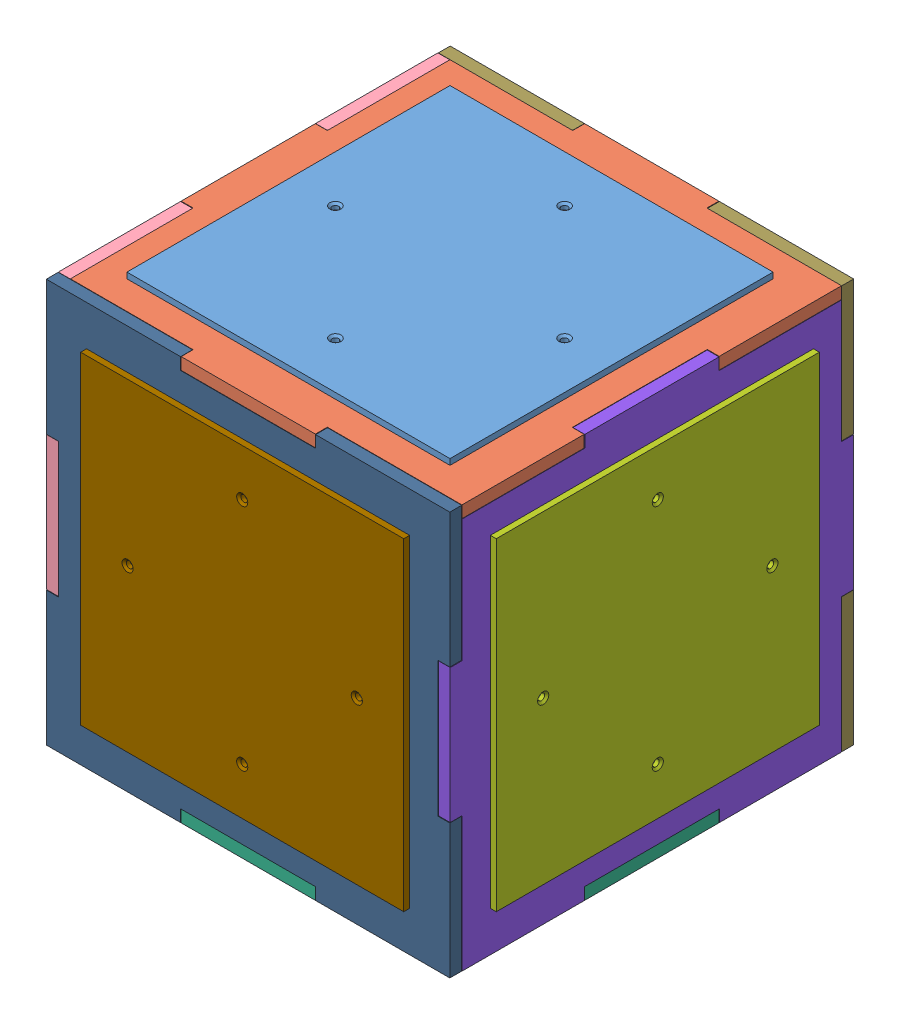
SolidWorks assembly cube_06, configuration cube06. Lengths in mm.
Overall size (112.39 112.39 116.4).
12 component instances, 12 part files, 6 mates.
Components (placement in the parent):
- panel_R^cube_06-13: panel_R^cube_06 [cube01] x (-1 0 0) z (0 0 1) (virtual)
- acrylic_R^cube_06-1: acrylic_R^cube_06 [A] at origin (virtual)
- panel_O^cube_06-8: panel_O^cube_06 [cube01] x (0 -1 0) z (0 0 1) (virtual)
- acrylic_O^cube_06-23: acrylic_O^cube_06 [A] x (0 1 0) z (0 0 1) (virtual)
- panel_Y^cube_06-9: panel_Y^cube_06 [cube01] at origin (virtual)
- acrylic_Y^cube_06-24: acrylic_Y^cube_06 [A] x (-1 0 0) z (0 0 1) (virtual)
- panel_G^cube_06-10: panel_G^cube_06 [cube01] x (0 1 0) z (0 0 1) (virtual)
- acrylic_G^cube_06-25: acrylic_G^cube_06 [A] x (0 -1 0) z (0 0 1) (virtual)
- panel_C^cube_06-11: panel_C^cube_06 [cube01] x (-1 0 0) z (0 -1 0) (virtual)
- acrylic_C^cube_06-26: acrylic_C^cube_06 [B] x (1 0 0) z (0 -1 0) (virtual)
- panel_B^cube_06-13: panel_B^cube_06 [cube01] x (-1 0 0) z (0 1 0) (virtual)
- acrylic_B^cube_06-27: acrylic_B^cube_06 [B] x (1 0 0) z (0 1 0) (virtual)
Mates (geometry in assembly coordinates):
- Coincident1: coincident aligned: plane of panel_R^cube_06-13 through (0 0 0) normal (0 0 1); plane of assembly through (0 0 0) normal (0 0 1)
- Coincident2: coincident anti-aligned: plane of panel_R^cube_06-13; plane of assembly through (0 0 0) normal (1 0 0)
- Coincident3: coincident anti-aligned: plane of panel_R^cube_06-13; plane of assembly through (0 0 0) normal (0 1 0)
- Coincident4: coincident aligned: plane of acrylic_R^cube_06-1 through (0 0 0) normal (0 0 1); plane of assembly through (0 0 0) normal (0 0 1)
- Coincident5: coincident aligned: plane of acrylic_R^cube_06-1 through (0 0 0) normal (1 0 0); plane of assembly through (0 0 0) normal (1 0 0)
- Coincident6: coincident aligned: plane of ? through (0 0 0) normal (0 1 0); plane of assembly through (0 0 0) normal (0 1 0)
